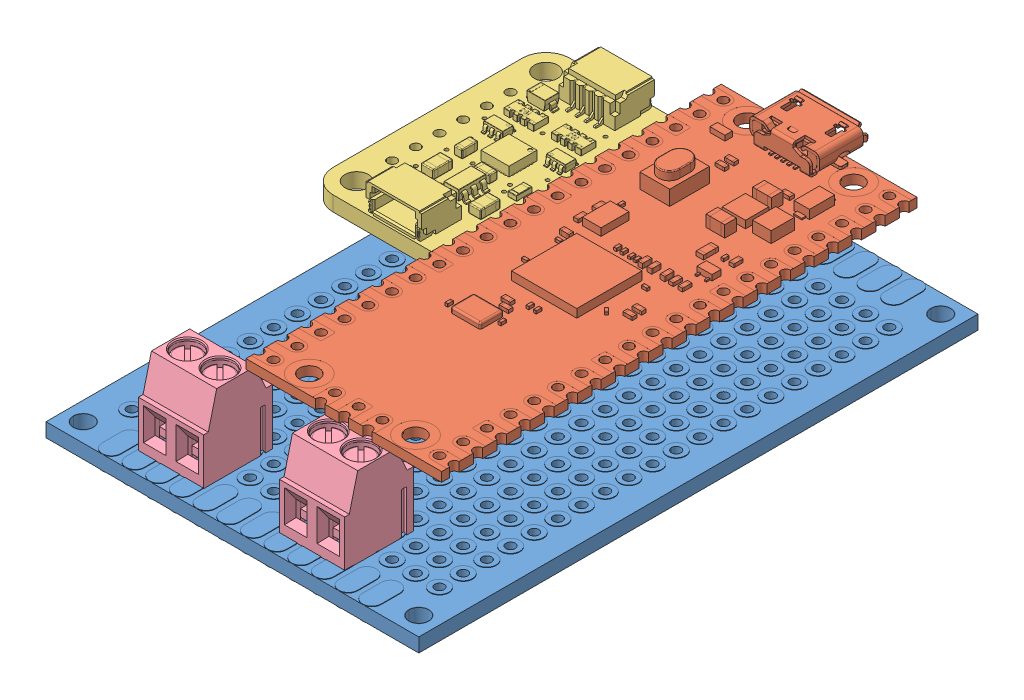
SolidWorks assembly Main_Board, configuration Default. Lengths in mm.
Overall size (44.13 18.54 60).
5 component instances, 4 part files, 8 mates.
Components (placement in the parent):
- Universal_board_40x60mm.stp-1: Universal_board_40x60mm.stp [Default] at origin size (40 1.6 60)
- Raspberry Pi Pico-R3-1: Raspberry Pi Pico-R3 [Default] at (-26.1161 13.25 58.3318) size (21 3.69 52.43)
- LSM6DSOX acc gyro-1: LSM6DSOX acc gyro [Default] at (-48.9661 4 43.0918) x (0 0 -1) z (0 1 0) size (25.4 17.78 4.55)
- PCB Terminal Block 2 DEG381-3.5.step-1: PCB Terminal Block 2 DEG381-3.5.step [Default] at (-44.2915 1.5 82.4428) x (1 0 0) z (0 1 0) size (7.4 7.4 12.2)
- PCB Terminal Block 2 DEG381-3.5.step-2: PCB Terminal Block 2 DEG381-3.5.step [Default] at (-29.0999 1.5 82.5034) x (1 0 0) z (0 1 0) size (7.4 7.4 12.2)
Mates (geometry in assembly coordinates):
- Concentric1: concentric anti-aligned: cylinder of Universal_board_40x60mm.stp-1 through (-17.2161 -0.05 82.4618) axis (0 -1 0) radius 0.5; cylinder of Raspberry Pi Pico-R3-1 through (-17.2161 13.75 82.4618) axis (0 1 0) radius 0.5
- Concentric2: concentric anti-aligned: cylinder of Universal_board_40x60mm.stp-1 through (-17.2161 -0.05 34.2018) axis (0 -1 0) radius 0.5; cylinder of Raspberry Pi Pico-R3-1 through (-17.2161 13.75 34.2018) axis (0 1 0) radius 0.5
- Distance1: distance = 11.25 mm anti-aligned: plane of Raspberry Pi Pico-R3-1 through (-26.1161 12.75 58.3318) normal (0 -1 0); plane of Universal_board_40x60mm.stp-1 through (-57.7261 1.5 94.1718) normal (0 1 0)
- Distance2: distance = 2.5 mm anti-aligned: plane of LSM6DSOX acc gyro-1 through (-48.9661 4 43.0918) normal (0 -1 0); plane of Universal_board_40x60mm.stp-1 through (-57.7261 1.5 94.1718) normal (0 1 0)
- Concentric3: concentric anti-aligned: cylinder of LSM6DSOX acc gyro-1 through (-42.6161 4 36.7418) axis (0 1 0) radius 0.5; cylinder of Universal_board_40x60mm.stp-1 through (-42.6161 -0.05 36.7418) axis (0 -1 0) radius 0.5
- Concentric4: concentric anti-aligned: cylinder of Universal_board_40x60mm.stp-1 through (-42.6161 -0.05 49.4418) axis (0 -1 0) radius 0.5; cylinder of LSM6DSOX acc gyro-1 through (-42.6161 4 49.4418) axis (0 1 0) radius 0.5
- Coincident3: coincident anti-aligned: plane of Universal_board_40x60mm.stp-1 through (-57.7261 1.5 94.1718) normal (0 1 0); plane of PCB Terminal Block 2 DEG381-3.5.step-1 through (-42.5744 1.5 82.0394) normal (0 -1 0)
- Coincident4: coincident anti-aligned: plane of Universal_board_40x60mm.stp-1 through (-57.7261 1.5 94.1718) normal (0 1 0); plane of PCB Terminal Block 2 DEG381-3.5.step-2 through (-27.3828 1.5 82.0999) normal (0 -1 0)
